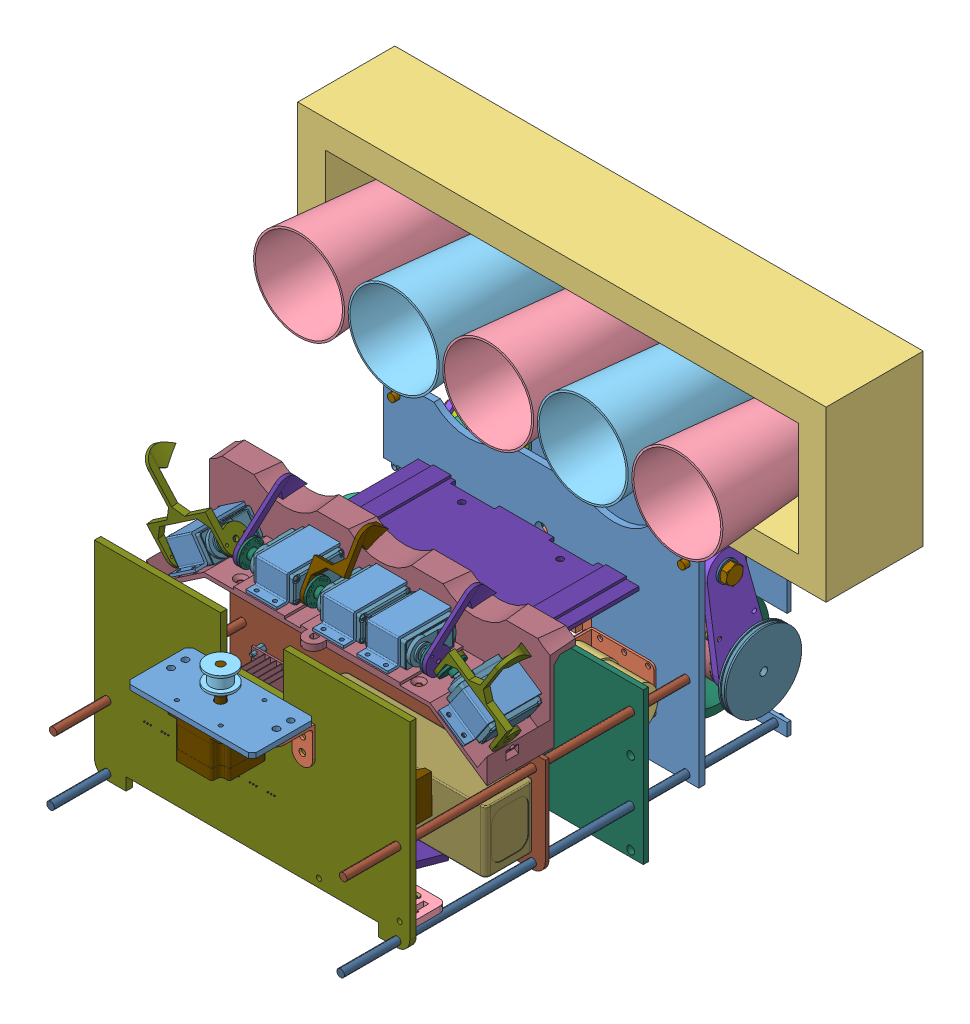
SolidWorks assembly Assemblage ROBOT SGHIR, configuration Default. Lengths in mm.
Overall size (419 329.19 386.9).
345 component instances, 73 part files, 218 mates.
Components (placement in the parent):
- baseee-1: baseee [Défaut] at (-18.9013 250.2954 189.5605) size (250 160 3)
- support_roulement-1: support_roulement [Défaut] at (62.0987 90.2954 212.5605) x (0 -1 0) z (1 0 0) size (45 40 8)
- support_roulement-2: support_roulement [Défaut] at (103.4987 90.2954 212.5605) x (0 1 0) z (-1 0 0) size (45 40 8)
- support_roulement-3: support_roulement [Défaut] at (150.0987 90.2954 212.5605) x (0 1 0) z (-1 0 0) size (45 40 8)
- support_roulement-4: support_roulement [Défaut] at (108.6987 90.2954 212.5605) x (0 1 0) z (1 0 0) size (45 40 8)
- roulement-1: roulement [Default] at (148.0987 90.2954 212.5605) x (0 0.989363 -0.145468) z (0 0.145468 0.989363) size (19 6 19)
- roulement-2: roulement [Default] at (116.6987 90.2954 212.5605) x (0 0.988428 -0.151694) z (0 0.151694 0.988428) size (19 6 19)
- roulement-3: roulement [Default] at (101.4987 90.2954 212.5605) x (0 0.989363 -0.145468) z (0 0.145468 0.989363) size (19 6 19)
- roulement-4: roulement [Default] at (70.0987 90.2954 212.5605) x (0 0.999601 -0.02823) z (0 0.02823 0.999601) size (19 6 19)
- axe de tombour-1: axe de tombour [Default] at (93.6516 90.2954 212.5605) x (0 -0.99338 -0.114871) z (-1 0 0) size (6 6 40)
- small_roue-1: small_roue [Défaut] at (80.1798 90.2954 212.5605) x (0 0.831954 -0.554845) z (1 0 0) size (23.1 23.1 19.4)
- axe de tombour-2: axe de tombour [Default] at (155.8668 90.2954 212.5605) x (0 -0.497154 0.867662) z (-1 0 0) size (6 6 40)
- small_roue-2: small_roue [Défaut] at (127.9937 90.2954 212.5605) x (0 0.856111 -0.516793) z (1 0 0) size (23.1 23.1 19.4)
- supportencodeur+encodeur+roue-1: supportencodeur+encodeur+roue [Default] at (226.6391 188.3182 195.4291) x (0 -1 0) z (-1 0 0) size (127.24 70.21 65.9)
  - Part1-1: Part1 [Default] at (40.5228 47.1314 27.8404) size (50 50 15)
  - axe-1: axe [Default] at (27.5228 27.1314 13.8404) x (0 0 -1) z (0.012333 0.999924 0) size (50 24 24)
  - levier-1: levier [Default] at (96.1154 13.1656 13.8404) x (0.979895 -0.199512 0) z (0 0 1) size (105 40 5)
  - hex screw gradeab fine_iso-1: hex screw gradeab fine_iso [ISO 8676 - M8x1.0 x 16-N] at (27.5228 27.1314 6.9404) x (0 0 1) z (0.127551 -0.991832 0) size (21.3 15.01 13)
  - plain washer normal grade a_iso-1: plain washer normal grade a_iso [Washer ISO 7089 - 8] at (27.5228 27.1314 13.8404) x (0 0 1) z (-0.997361 0.072597 0) size (1.6 16 16)
  - socket head cap screw_iso-5: socket head cap screw_iso [ISO 4762 M3 x 8 - 8N] at (27.7694 47.1299 22.3404) x (-0.012333 -0.999924 0) z (-0.32391 0.003995 0.946079) size (11 5.5 5.5)
  - socket head cap screw_iso-6: socket head cap screw_iso [ISO 4762 M3 x 8 - 8N] at (7.5243 27.3781 22.3404) x (0.999924 -0.012333 0) z (0.005971 0.484095 0.874995) size (11 5.5 5.5)
  - slotted pan head screw_iso-1: slotted pan head screw_iso [ISO 1580 - M4 x 5 - 5N] at (72.2121 32.4102 22.2404) x (0 0 -1) z (-0.691437 -0.722437 0) size (7.47 8 8)
  - Encodeur TR-1: Encodeur TR [Défaut] at (96.1154 13.1656 54.4404) x (0.979895 -0.199512 0) z (0 0 -1) size (37.8 37.8 52.6)
  - Roue Encodeur-1: Roue Encodeur [Défaut] at (96.1154 13.1656 3.9404) x (0 0 -1) z (-0.130263 -0.99148 0) size (14 60 60)
  - socket head cap screw_iso-7: socket head cap screw_iso [ISO 4762 M4 x 30 - 20N] at (14.9228 40.1314 35.4102) x (1 0 0) z (0 -0.701601 -0.71257) size (34 7 7)
- Tombour-1: Tombour [Défaut] at (165.0768 90.2954 212.5605) x (-1 0 0) z (0 0.352359 -0.935865) size (40 84.84 84.84)
- Motor Cople-1: Motor Cople [Predeterminado] at (152.8668 90.2954 212.5605) x (0 0 1) z (-1 0 0) size (25.4 25.4 9.21)
- Tombour + levier gauche-2: Tombour + levier gauche [Défaut] at (130.7568 41.7681 187.0189) x (-1 0 0) z (0 1 0) size (65.9 83.26 124.85)
  - supportencodeur+encodeur+roue-1: supportencodeur+encodeur+roue [Default] at (145.1984 8.4101 91.5046) x (0 0 1) z (-1 0 0) size (124.85 83.26 65.9) (flexible)
    - Part1-1: Part1 [Default] at (40.5228 47.1314 27.8404) size (50 50 15)
    - axe-1: axe [Default] at (27.5228 27.1314 13.8404) x (0 0 -1) z (0.999994 0.003586 0) size (50 24 24)
    - levier-1: levier [Default] at (-37.9241 2.2978 13.8404) x (-0.934955 -0.354766 0) z (0 0 1) size (105 40 5)
    - hex screw gradeab fine_iso-1: hex screw gradeab fine_iso [ISO 8676 - M8x1.0 x 16-N] at (27.5228 27.1314 6.9404) x (0 0 1) z (0.924079 -0.382202 0) size (21.3 15.01 13)
    - plain washer normal grade a_iso-1: plain washer normal grade a_iso [Washer ISO 7089 - 8] at (27.5228 27.1314 13.8404) x (0 0 1) z (-0.973268 0.229671 0) size (1.6 16 16)
    - socket head cap screw_iso-5: socket head cap screw_iso [ISO 4762 M3 x 8 - 8N] at (47.5226 27.2031 22.3404) x (-0.999994 -0.003586 0) z (-0.003073 0.857033 -0.515253) size (11 5.5 5.5)
    - socket head cap screw_iso-6: socket head cap screw_iso [ISO 4762 M3 x 8 - 8N] at (27.451 47.1313 22.3404) x (0.003586 -0.999994 0) z (0.889754 0.00319 0.45643) size (11 5.5 5.5)
    - slotted pan head screw_iso-1: slotted pan head screw_iso [ISO 1580 - M4 x 5 - 5N] at (-7.4369 -1.2027 22.2404) x (0 0 -1) z (0.467296 0.884101 0) size (7.47 8 8)
    - Encodeur TR-1: Encodeur TR [Défaut] at (-37.9241 2.2978 54.4404) x (-0.934955 -0.354766 0) z (0 0 -1) size (37.8 37.8 52.6)
    - Roue Encodeur-1: Roue Encodeur [Défaut] at (-37.9241 2.2978 3.9404) x (0 0 -1) z (0.159731 -0.987161 0) size (14 60 60)
    - socket head cap screw_iso-7: socket head cap screw_iso [ISO 4762 M4 x 30 - 20N] at (14.9228 40.1314 35.4102) x (1 0 0) z (0 -0.489793 0.871839) size (34 7 7)
- Tombour-2: Tombour [Défaut] at (47.3307 90.2954 212.5605) x (1 0 0) z (0 -0.872139 0.489257) size (40 84.84 84.84)
- accouplement moteur-1: accouplement moteur [Défaut] at (50.3307 90.2954 212.5605) size (9 25 25)
- scroll 04-1: scroll 04 [Défaut] at (77.2489 172.6222 180.1625) x (-0.291584 0.956545 0) z (0 0 1) size (20.32 14.73 13.46)
- etage moutourat-1: etage moutourat [Défaut] at (-18.9013 200.2954 257.5605) size (250 160 5)
- moteurKacem+support-1: moteurKacem+support [Default] at (34.6337 134.2418 250.1858) x (1 0 0) z (0 -1 0) size (79.5 40.7 38)
  - supportMoteur-1: supportMoteur [Default] at (29.6651 14.0747 22.9463) size (51 40.7 38)
  - moteurKacem-1: moteurKacem [Default] at (5.9651 33.0886 41.927) x (-1 0 0) z (0 -0.002768 -0.999996) size (79.5 37 37)
- support servo allu-2: support servo allu [Default] at (0.5987 137.4885 257.5605) x (1 0 0) z (0 1 0) size (80 24 5)
- moteurKacem+support-2: moteurKacem+support [Default] at (177.5638 47.8491 250.1858) x (-1 0 0) z (0 1 0) size (79.5 40.7 38)
  - supportMoteur-1: supportMoteur [Default] at (29.6651 14.0747 22.9463) size (51 40.7 38)
  - moteurKacem-1: moteurKacem [Default] at (5.9651 33.0886 41.927) x (-1 0 0) z (0 -0.002768 -0.999996) size (79.5 37 37)
- ServoAttacment2-1: ServoAttacment2 [Varsayılan] at (31.0987 127.0525 248.5605) x (0.695152 0 0.718863) z (0 -1 0) size (14 25.75 6.08)
- bras manche a air-1: bras manche a air [Default] at (28.9422 121.0525 250.6459) x (-0.718863 0 0.695152) z (0 1 0) size (80 30 4)
- small_roue-3: small_roue [Défaut] at (132.8487 89.7954 276.2744) x (0 0.856111 -0.516793) z (1 0 0) size (23.1 23.1 19.4)
- small_roue-4: small_roue [Défaut] at (79.3487 92.2954 276.2744) x (0 0.830482 -0.557045) z (-1 0 0) size (23.1 23.1 19.4)
- vis fixation tambour-1: vis fixation tambour [Default] at (66.0987 72.7954 257.5605) x (1 0 0) z (0 1 0) size (5 69.8 5)
- vis fixation tambour-2: vis fixation tambour [Default] at (66.0987 107.7954 257.5605) x (1 0 0) z (0 1 0) size (5 69.8 5)
- vis fixation tambour-3: vis fixation tambour [Default] at (99.4987 72.7954 257.5605) x (1 0 0) z (0 1 0) size (5 69.8 5)
- vis fixation tambour-4: vis fixation tambour [Default] at (99.4987 107.7954 257.5605) x (1 0 0) z (0 1 0) size (5 69.8 5)
- ressort-1: ressort [Default] at (64.5295 107.7954 230.9339) size (4.4 5.08 25.07)
- ressort-2: ressort [Default] at (97.9295 107.8027 231.9339) x (0.999989 -0.004615 0) z (0 0 1) size (4.4 5.08 25.07)
- ressort-3: ressort [Default] at (97.9295 72.8027 231.9339) x (0.999989 -0.004615 0) z (0 0 1) size (4.4 5.08 25.07)
- ressort-4: ressort [Default] at (64.5295 72.7954 235.9339) size (4.4 5.08 25.07)
- ressort-5: ressort [Default] at (111.1295 72.8027 231.9339) x (0.999989 -0.004615 0) z (0 0 1) size (4.4 5.08 25.07)
- vis fixation tambour-5: vis fixation tambour [Default] at (112.6987 107.7954 257.5605) x (1 0 0) z (0 1 0) size (5 69.8 5)
- vis fixation tambour-6: vis fixation tambour [Default] at (112.6987 72.7954 257.5605) x (1 0 0) z (0 1 0) size (5 69.8 5)
- vis fixation tambour-7: vis fixation tambour [Default] at (146.0987 72.7954 257.5605) x (1 0 0) z (0 1 0) size (5 69.8 5)
- vis fixation tambour-8: vis fixation tambour [Default] at (146.0987 107.7954 257.5605) x (1 0 0) z (0 1 0) size (5 69.8 5)
- ressort-6: ressort [Default] at (113.6444 106.5431 231.9339) x (-0.602601 0.798042 0) z (0 0 1) size (4.4 5.08 25.07)
- ressort-7: ressort [Default] at (147.0444 106.5431 231.9339) x (-0.602601 0.798042 0) z (0 0 1) size (4.4 5.08 25.07)
- ressort-8: ressort [Default] at (147.0444 71.5431 231.9339) x (-0.602601 0.798042 0) z (0 0 1) size (4.4 5.08 25.07)
- salim écrou-1: salim écrou [Défaut] at (65.7102 107.8336 251.7883) x (-0.68705 0.72661 0) z (0 0 1) size (5.79 5.76 11.17)
- rondelle-1: rondelle [Default] at (66.0987 107.7954 253.0605) size (9 9 0.5)
- 3 etage-1: 3 etage [Default] at (-18.9013 120.2954 381.2939) size (250 80 3)
- Lipot 5000 mAh-1: Lipot 5000 mAh [Default] at (153.6734 75.7626 399.2939) size (150 49 39)
- L298N Motor Driver-1: L298N Motor Driver [Default] at (26.3982 67.0454 389.2939) x (-1 0 0) z (0 1 0) size (43.5 26 43.5)
- entretoise-1: entretoise [Default] at (7.5152 85.7854 389.2939) x (0 0 -1) z (0.075316 -0.99716 0) size (10.06 5.77 5)
- entretoise-2: entretoise [Default] at (45.0327 48.3621 389.2939) x (0 0 -1) z (-0.5 -0.866025 0) size (10.06 5.77 5)
- entretoise-3: entretoise [Default] at (7.7636 48.3621 389.2939) x (0 0 -1) z (-0.5 0.866025 0) size (10.06 5.77 5)
- entretoise-4: entretoise [Default] at (45.0152 85.7854 389.2939) x (0 0 -1) z (0.075316 -0.99716 0) size (10.06 5.77 5)
- étage servo-1: étage servo [Default] at (-18.9013 129.7933 302.5605) size (250 120 4)
- etage electro-1: etage electro [Défaut] at (231.0987 40.2954 486.706) x (-1 0 0) z (0 0 1) size (250 160 5)
- support servo allu-3: support servo allu [Default] at (170.5987 56.9278 486.706) x (1 0 0) z (0 1 0) size (80 24 5)
- 3alam-1: 3alam [Défaut] at (66.7107 40.2954 431.5663) x (0.357807 0 -0.933796) z (0 1 0) size (60 150 5)
- ServoAttacment2-3: ServoAttacment2 [Varsayılan] at (201.0987 47.2954 477.706) x (-0.357807 0 0.933796) z (0 -1 0) size (14 25.75 6.08)
- TB6560 Stepper driver-1: TB6560 Stepper driver [Default] at (173.9926 122.1069 469.706) x (-0.019439 0.999811 0) z (0.999811 0.019439 0) size (50 34 75)
- Carte 8 servos.STEP-1: Carte 8 servos.STEP [Default] at (127.4764 76.1908 483.471) x (-1 0 0) z (0 0 -1) size (135 60 28.62)
  - U1.STEP-1: U1.STEP [Default] at (2.3 7.3 0.775) x (0 -1 0) z (0 0 1) size (7.62 7.92 7.75)
    - Open CASCADE STEP translator 6.8 2.2.1.STEP-1: Open CASCADE STEP translator 6.8 2.2.1.STEP [Default] at origin size (7.62 7.92 7.75)
      - Body_1.STEP-1: Body_1.STEP [Default] at (2.5 4 0) x (0 1 0) z (1 0 0) size (7.92 7.75 7.62)
  - U2.STEP-1: U2.STEP [Default] at (16.56 8.1 0.775) x (0 -1 0) z (0 0 1) size (7.62 7.92 7.75)
    - Open CASCADE STEP translator 6.8 2.3.1.STEP-1: Open CASCADE STEP translator 6.8 2.3.1.STEP [Default] at origin size (7.62 7.92 7.75)
      - Body_1.STEP-1: Body_1.STEP [Default] at (2.5 4 0) x (0 1 0) z (1 0 0) size (7.92 7.75 7.62)
  - U3.STEP-1: U3.STEP [Default] at (30.3 7.8 0.775) x (0 -1 0) z (0 0 1) size (7.62 7.92 7.75)
    - Open CASCADE STEP translator 6.8 2.4.1.STEP-1: Open CASCADE STEP translator 6.8 2.4.1.STEP [Default] at origin size (7.62 7.92 7.75)
      - Body_1.STEP-1: Body_1.STEP [Default] at (2.5 4 0) x (0 1 0) z (1 0 0) size (7.92 7.75 7.62)
  - U4.STEP-1: U4.STEP [Default] at (44.2 7.6 0.775) x (0 -1 0) z (0 0 1) size (7.62 7.92 7.75)
    - Open CASCADE STEP translator 6.8 2.5.1.STEP-1: Open CASCADE STEP translator 6.8 2.5.1.STEP [Default] at origin size (7.62 7.92 7.75)
      - Body_1.STEP-1: Body_1.STEP [Default] at (2.5 4 0) x (0 1 0) z (1 0 0) size (7.92 7.75 7.62)
  - J2.STEP-1: J2.STEP [Default] at (9.1 -11.4 0.775) x (-1 0 0) z (0 0 1) size (6 2 8.8)
    - Open CASCADE STEP translator 6.8 2.6.1.STEP-1: Open CASCADE STEP translator 6.8 2.6.1.STEP [Default] at origin size (6 2 8.8)
      - Body_1-0.STEP-1: Body_1-0.STEP [Default] at (1.5 -1 -3) x (0 1 0) z (1 0 0) size (2 8.8 6)
        - Carte 8 servos-prt1.STEP-1: Carte 8 servos-prt1.STEP [Default] at origin size (2 8.8 2)
        - Carte 8 servos-prt2.STEP-1: Carte 8 servos-prt2.STEP [Default] at origin size (2 8.8 2)
        - Carte 8 servos-prt3.STEP-1: Carte 8 servos-prt3.STEP [Default] at origin size (2 8.8 2)
  - J3.STEP-1: J3.STEP [Default] at (22.86 -11.3 0.775) x (-1 0 0) z (0 0 1) size (6 2 8.8)
    - Open CASCADE STEP translator 6.8 2.7.1.STEP-1: Open CASCADE STEP translator 6.8 2.7.1.STEP [Default] at origin size (6 2 8.8)
      - Body_1-0.STEP-1: Body_1-0.STEP [Default] at (1.5 -1 -3) x (0 1 0) z (1 0 0) size (2 8.8 6)
        - Carte 8 servos-prt1.STEP-1: Carte 8 servos-prt1.STEP [Default] at origin size (2 8.8 2)
        - Carte 8 servos-prt2.STEP-1: Carte 8 servos-prt2.STEP [Default] at origin size (2 8.8 2)
        - Carte 8 servos-prt3.STEP-1: Carte 8 servos-prt3.STEP [Default] at origin size (2 8.8 2)
  - J4.STEP-1: J4.STEP [Default] at (36.8 -11.3 0.775) x (-1 0 0) z (0 0 1) size (6 2 8.8)
    - Open CASCADE STEP translator 6.8 2.8.1.STEP-1: Open CASCADE STEP translator 6.8 2.8.1.STEP [Default] at origin size (6 2 8.8)
      - Body_1-0.STEP-1: Body_1-0.STEP [Default] at (1.5 -1 -3) x (0 1 0) z (1 0 0) size (2 8.8 6)
        - Carte 8 servos-prt1.STEP-1: Carte 8 servos-prt1.STEP [Default] at origin size (2 8.8 2)
        - Carte 8 servos-prt2.STEP-1: Carte 8 servos-prt2.STEP [Default] at origin size (2 8.8 2)
        - Carte 8 servos-prt3.STEP-1: Carte 8 servos-prt3.STEP [Default] at origin size (2 8.8 2)
  - J5.STEP-1: J5.STEP [Default] at (50.7 -11.3 0.775) x (-1 0 0) z (0 0 1) size (6 2 8.8)
    - Open CASCADE STEP translator 6.8 2.9.1.STEP-1: Open CASCADE STEP translator 6.8 2.9.1.STEP [Default] at origin size (6 2 8.8)
      - Body_1-0.STEP-1: Body_1-0.STEP [Default] at (1.5 -1 -3) x (0 1 0) z (1 0 0) size (2 8.8 6)
        - Carte 8 servos-prt1.STEP-1: Carte 8 servos-prt1.STEP [Default] at origin size (2 8.8 2)
        - Carte 8 servos-prt2.STEP-1: Carte 8 servos-prt2.STEP [Default] at origin size (2 8.8 2)
        - Carte 8 servos-prt3.STEP-1: Carte 8 servos-prt3.STEP [Default] at origin size (2 8.8 2)
  - J6.STEP-1: J6.STEP [Default] at (-4.8 19.8 0.775) x (-1 0 0) z (0 0 1) size (10 7.5 13.25)
    - Open CASCADE STEP translator 6.8 2.10.1.STEP-1: Open CASCADE STEP translator 6.8 2.10.1.STEP [Default] at origin size (10 7.5 13.25)
      - Body_1-1.STEP-1: Body_1-1.STEP [Default] at (7.5 4 0) x (-1 0 0) z (0 1 0) size (10 13.25 7.5)
  - C1.STEP-1: C1.STEP [Default] at (-5.9 9.4 0.775) x (-1 0 0) z (0 0 1) size (6.31 6.3 13.91)
    - Open CASCADE STEP translator 6.8 2.11.1.STEP-1: Open CASCADE STEP translator 6.8 2.11.1.STEP [Default] at origin size (6.31 6.3 13.91)
      - Body_1-2.STEP-1: Body_1-2.STEP [Default] at (1.25 0 0) x (1 0 0) z (0 -1 0) size (6.31 13.91 6.3)
  - C9.STEP-1: C9.STEP [Default] at (7.54 -3.5 0.775) x (-1 0 0) z (0 0 1) size (6.31 6.3 13.91)
    - Open CASCADE STEP translator 6.8 2.12.1.STEP-1: Open CASCADE STEP translator 6.8 2.12.1.STEP [Default] at origin size (6.31 6.3 13.91)
      - Body_1-2.STEP-1: Body_1-2.STEP [Default] at (1.25 0 0) x (1 0 0) z (0 -1 0) size (6.31 13.91 6.3)
  - C10.STEP-1: C10.STEP [Default] at (21.36 -2.9 0.775) x (-1 0 0) z (0 0 1) size (6.31 6.3 13.91)
    - Open CASCADE STEP translator 6.8 2.13.1.STEP-1: Open CASCADE STEP translator 6.8 2.13.1.STEP [Default] at origin size (6.31 6.3 13.91)
      - Body_1-2.STEP-1: Body_1-2.STEP [Default] at (1.25 0 0) x (1 0 0) z (0 -1 0) size (6.31 13.91 6.3)
  - C11.STEP-1: C11.STEP [Default] at (35.5 -2.8 0.775) x (-1 0 0) z (0 0 1) size (6.31 6.3 13.91)
    - Open CASCADE STEP translator 6.8 2.14.1.STEP-1: Open CASCADE STEP translator 6.8 2.14.1.STEP [Default] at origin size (6.31 6.3 13.91)
      - Body_1-2.STEP-1: Body_1-2.STEP [Default] at (1.25 0 0) x (1 0 0) z (0 -1 0) size (6.31 13.91 6.3)
  - C12.STEP-1: C12.STEP [Default] at (49.2 -3 0.775) x (-1 0 0) z (0 0 1) size (6.31 6.3 13.91)
    - Open CASCADE STEP translator 6.8 2.15.1.STEP-1: Open CASCADE STEP translator 6.8 2.15.1.STEP [Default] at origin size (6.31 6.3 13.91)
      - Body_1-2.STEP-1: Body_1-2.STEP [Default] at (1.25 0 0) x (1 0 0) z (0 -1 0) size (6.31 13.91 6.3)
  - R1.STEP-1: R1.STEP [Default] at (11.2 11.3 0.775) x (-1 0 0) z (0 0 1) size (10.82 1.37 5.33)
    - Open CASCADE STEP translator 6.8 2.16.1.STEP-1: Open CASCADE STEP translator 6.8 2.16.1.STEP [Default] at origin size (10.82 1.37 5.33)
      - Body_1-3.STEP-1: Body_1-3.STEP [Default] at origin size (5.08 1.37 1.37)
      - Pin_1.STEP-1: Pin_1.STEP [Default] at origin size (3.2 0.66 4.98)
      - Pin_2.STEP-1: Pin_2.STEP [Default] at (20.32 0 0) x (-1 0 0) z (0 0 1) size (3.2 0.66 4.98)
  - R2.STEP-1: R2.STEP [Default] at (25.16 11.3 0.775) x (-1 0 0) z (0 0 1) size (10.82 1.37 5.33)
    - Open CASCADE STEP translator 6.8 2.16.1.STEP-1: Open CASCADE STEP translator 6.8 2.16.1.STEP [Default] at origin size (10.82 1.37 5.33)
      - Body_1-3.STEP-1: Body_1-3.STEP [Default] at origin size (5.08 1.37 1.37)
      - Pin_1.STEP-1: Pin_1.STEP [Default] at origin size (3.2 0.66 4.98)
      - Pin_2.STEP-1: Pin_2.STEP [Default] at (20.32 0 0) x (-1 0 0) z (0 0 1) size (3.2 0.66 4.98)
  - R3.STEP-1: R3.STEP [Default] at (28.8 11 0.775) size (10.82 1.37 5.33)
    - Open CASCADE STEP translator 6.8 2.16.1.STEP-1: Open CASCADE STEP translator 6.8 2.16.1.STEP [Default] at origin size (10.82 1.37 5.33)
      - Body_1-3.STEP-1: Body_1-3.STEP [Default] at origin size (5.08 1.37 1.37)
      - Pin_1.STEP-1: Pin_1.STEP [Default] at origin size (3.2 0.66 4.98)
      - Pin_2.STEP-1: Pin_2.STEP [Default] at (20.32 0 0) x (-1 0 0) z (0 0 1) size (3.2 0.66 4.98)
  - R4.STEP-1: R4.STEP [Default] at (53.56 11.6 0.775) x (-1 0 0) z (0 0 1) size (10.82 1.37 5.33)
    - Open CASCADE STEP translator 6.8 2.16.1.STEP-1: Open CASCADE STEP translator 6.8 2.16.1.STEP [Default] at origin size (10.82 1.37 5.33)
      - Body_1-3.STEP-1: Body_1-3.STEP [Default] at origin size (5.08 1.37 1.37)
      - Pin_1.STEP-1: Pin_1.STEP [Default] at origin size (3.2 0.66 4.98)
      - Pin_2.STEP-1: Pin_2.STEP [Default] at (20.32 0 0) x (-1 0 0) z (0 0 1) size (3.2 0.66 4.98)
  - U6.STEP-1: U6.STEP [Default] at (48.34 19.4 0.775) size (9.97 4.45 28.62)
    - Open CASCADE STEP translator 6.8 2.20.1.STEP-1: Open CASCADE STEP translator 6.8 2.20.1.STEP [Default] at origin size (9.97 4.45 28.62)
      - Body_1-4.STEP-1: Body_1-4.STEP [Default] at (0 3 3.5) x (1 0 0) z (0 -1 0) size (9.97 28.62 4.45)
  - U7.STEP-1: U7.STEP [Default] at (20.1 19.4 0.775) size (9.97 4.45 28.62)
    - Open CASCADE STEP translator 6.8 2.21.1.STEP-1: Open CASCADE STEP translator 6.8 2.21.1.STEP [Default] at origin size (9.97 4.45 28.62)
      - Body_1-4.STEP-1: Body_1-4.STEP [Default] at (0 3 3.5) x (1 0 0) z (0 -1 0) size (9.97 28.62 4.45)
  - U8.STEP-1: U8.STEP [Default] at (34.14 19.2 0.775) size (9.97 4.45 28.62)
    - Open CASCADE STEP translator 6.8 2.22.1.STEP-1: Open CASCADE STEP translator 6.8 2.22.1.STEP [Default] at origin size (9.97 4.45 28.62)
      - Body_1-4.STEP-1: Body_1-4.STEP [Default] at (0 3 3.5) x (1 0 0) z (0 -1 0) size (9.97 28.62 4.45)
  - U5.STEP-1: U5.STEP [Default] at (5.9 19.8 0.775) size (9.97 4.45 28.62)
    - Open CASCADE STEP translator 6.8 2.23.1.STEP-1: Open CASCADE STEP translator 6.8 2.23.1.STEP [Default] at origin size (9.97 4.45 28.62)
      - Body_1-4.STEP-1: Body_1-4.STEP [Default] at (0 3 3.5) x (1 0 0) z (0 -1 0) size (9.97 28.62 4.45)
  - D1.STEP-1: D1.STEP [Default] at (0.84 15.5 0.775) size (11.02 2.72 5.32)
    - Open CASCADE STEP translator 6.8 2.24.1.STEP-1: Open CASCADE STEP translator 6.8 2.24.1.STEP [Default] at origin size (11.02 2.72 5.32)
      - Body_1-5.STEP-1: Body_1-5.STEP [Default] at (10.1 0 0) size (11.02 2.72 5.32)
  - D2.STEP-1: D2.STEP [Default] at (15.4 15.3 0.775) size (11.02 2.72 5.32)
    - Open CASCADE STEP translator 6.8 2.25.1.STEP-1: Open CASCADE STEP translator 6.8 2.25.1.STEP [Default] at origin size (11.02 2.72 5.32)
      - Body_1-5.STEP-1: Body_1-5.STEP [Default] at (10.1 0 0) size (11.02 2.72 5.32)
  - D4.STEP-1: D4.STEP [Default] at (43 15.3 0.775) size (11.02 2.72 5.32)
    - Open CASCADE STEP translator 6.8 2.26.1.STEP-1: Open CASCADE STEP translator 6.8 2.26.1.STEP [Default] at origin size (11.02 2.72 5.32)
      - Body_1-5.STEP-1: Body_1-5.STEP [Default] at (10.1 0 0) size (11.02 2.72 5.32)
  - D3.STEP-1: D3.STEP [Default] at (29.24 15 0.775) size (11.02 2.72 5.32)
    - Open CASCADE STEP translator 6.8 2.27.1.STEP-1: Open CASCADE STEP translator 6.8 2.27.1.STEP [Default] at origin size (11.02 2.72 5.32)
      - Body_1-5.STEP-1: Body_1-5.STEP [Default] at (10.1 0 0) size (11.02 2.72 5.32)
  - U13.STEP-1: U13.STEP [Default] at (61.94 19.4 0.775) size (9.97 4.45 28.62)
    - Open CASCADE STEP translator 6.8 2.28.1.STEP-1: Open CASCADE STEP translator 6.8 2.28.1.STEP [Default] at origin size (9.97 4.45 28.62)
      - Body_1-4.STEP-1: Body_1-4.STEP [Default] at (0 3 3.5) x (1 0 0) z (0 -1 0) size (9.97 28.62 4.45)
  - U14.STEP-1: U14.STEP [Default] at (75.94 19.4 0.775) size (9.97 4.45 28.62)
    - Open CASCADE STEP translator 6.8 2.29.1.STEP-1: Open CASCADE STEP translator 6.8 2.29.1.STEP [Default] at origin size (9.97 4.45 28.62)
      - Body_1-4.STEP-1: Body_1-4.STEP [Default] at (0 3 3.5) x (1 0 0) z (0 -1 0) size (9.97 28.62 4.45)
  - U16.STEP-1: U16.STEP [Default] at (90.04 19.3 0.775) size (9.97 4.45 28.62)
    - Open CASCADE STEP translator 6.8 2.30.1.STEP-1: Open CASCADE STEP translator 6.8 2.30.1.STEP [Default] at origin size (9.97 4.45 28.62)
      - Body_1-4.STEP-1: Body_1-4.STEP [Default] at (0 3 3.5) x (1 0 0) z (0 -1 0) size (9.97 28.62 4.45)
  - U15.STEP-1: U15.STEP [Default] at (103.94 19.2 0.775) size (9.97 4.45 28.62)
    - Open CASCADE STEP translator 6.8 2.31.1.STEP-1: Open CASCADE STEP translator 6.8 2.31.1.STEP [Default] at origin size (9.97 4.45 28.62)
      - Body_1-4.STEP-1: Body_1-4.STEP [Default] at (0 3 3.5) x (1 0 0) z (0 -1 0) size (9.97 28.62 4.45)
  - D8.STEP-1: D8.STEP [Default] at (57.3 15.2 0.775) size (11.02 2.72 5.32)
    - Open CASCADE STEP translator 6.8 2.32.1.STEP-1: Open CASCADE STEP translator 6.8 2.32.1.STEP [Default] at origin size (11.02 2.72 5.32)
      - Body_1-5.STEP-1: Body_1-5.STEP [Default] at (10.1 0 0) size (11.02 2.72 5.32)
  - U9.STEP-1: U9.STEP [Default] at (58.8 7.9 0.775) x (0 -1 0) z (0 0 1) size (7.62 7.92 7.75)
    - Open CASCADE STEP translator 6.8 2.33.1.STEP-1: Open CASCADE STEP translator 6.8 2.33.1.STEP [Default] at origin size (7.62 7.92 7.75)
      - Body_1.STEP-1: Body_1.STEP [Default] at (2.5 4 0) x (0 1 0) z (1 0 0) size (7.92 7.75 7.62)
  - R5.STEP-1: R5.STEP [Default] at (57.3 11.4 0.775) size (10.82 1.37 5.33)
    - Open CASCADE STEP translator 6.8 2.16.1.STEP-1: Open CASCADE STEP translator 6.8 2.16.1.STEP [Default] at origin size (10.82 1.37 5.33)
      - Body_1-3.STEP-1: Body_1-3.STEP [Default] at origin size (5.08 1.37 1.37)
      - Pin_1.STEP-1: Pin_1.STEP [Default] at origin size (3.2 0.66 4.98)
      - Pin_2.STEP-1: Pin_2.STEP [Default] at (20.32 0 0) x (-1 0 0) z (0 0 1) size (3.2 0.66 4.98)
  - C2.STEP-1: C2.STEP [Default] at (64.04 -2.9 0.775) x (-1 0 0) z (0 0 1) size (6.31 6.3 13.91)
    - Open CASCADE STEP translator 6.8 2.35.1.STEP-1: Open CASCADE STEP translator 6.8 2.35.1.STEP [Default] at origin size (6.31 6.3 13.91)
      - Body_1-2.STEP-1: Body_1-2.STEP [Default] at (1.25 0 0) x (1 0 0) z (0 -1 0) size (6.31 13.91 6.3)
  - J7.STEP-1: J7.STEP [Default] at (65.5 -11.3 0.775) x (-1 0 0) z (0 0 1) size (6 2 8.8)
    - Open CASCADE STEP translator 6.8 2.36.1.STEP-1: Open CASCADE STEP translator 6.8 2.36.1.STEP [Default] at origin size (6 2 8.8)
      - Body_1-0.STEP-1: Body_1-0.STEP [Default] at (1.5 -1 -3) x (0 1 0) z (1 0 0) size (2 8.8 6)
        - Carte 8 servos-prt1.STEP-1: Carte 8 servos-prt1.STEP [Default] at origin size (2 8.8 2)
        - Carte 8 servos-prt2.STEP-1: Carte 8 servos-prt2.STEP [Default] at origin size (2 8.8 2)
        - Carte 8 servos-prt3.STEP-1: Carte 8 servos-prt3.STEP [Default] at origin size (2 8.8 2)
  - D5.STEP-1: D5.STEP [Default] at (99.4 14.7 0.775) size (11.02 2.72 5.32)
    - Open CASCADE STEP translator 6.8 2.37.1.STEP-1: Open CASCADE STEP translator 6.8 2.37.1.STEP [Default] at origin size (11.02 2.72 5.32)
      - Body_1-5.STEP-1: Body_1-5.STEP [Default] at (10.1 0 0) size (11.02 2.72 5.32)
  - D6.STEP-1: D6.STEP [Default] at (85.1 14.8 0.775) size (11.02 2.72 5.32)
    - Open CASCADE STEP translator 6.8 2.38.1.STEP-1: Open CASCADE STEP translator 6.8 2.38.1.STEP [Default] at origin size (11.02 2.72 5.32)
      - Body_1-5.STEP-1: Body_1-5.STEP [Default] at (10.1 0 0) size (11.02 2.72 5.32)
  - D7.STEP-1: D7.STEP [Default] at (71.24 14.8 0.775) size (11.02 2.72 5.32)
    - Open CASCADE STEP translator 6.8 2.39.1.STEP-1: Open CASCADE STEP translator 6.8 2.39.1.STEP [Default] at origin size (11.02 2.72 5.32)
      - Body_1-5.STEP-1: Body_1-5.STEP [Default] at (10.1 0 0) size (11.02 2.72 5.32)
  - R6.STEP-1: R6.STEP [Default] at (71.4 11.4 0.775) size (10.82 1.37 5.33)
    - Open CASCADE STEP translator 6.8 2.16.1.STEP-1: Open CASCADE STEP translator 6.8 2.16.1.STEP [Default] at origin size (10.82 1.37 5.33)
      - Body_1-3.STEP-1: Body_1-3.STEP [Default] at origin size (5.08 1.37 1.37)
      - Pin_1.STEP-1: Pin_1.STEP [Default] at origin size (3.2 0.66 4.98)
      - Pin_2.STEP-1: Pin_2.STEP [Default] at (20.32 0 0) x (-1 0 0) z (0 0 1) size (3.2 0.66 4.98)
  - R7.STEP-1: R7.STEP [Default] at (84.8 11.2 0.775) size (10.82 1.37 5.33)
    - Open CASCADE STEP translator 6.8 2.16.1.STEP-1: Open CASCADE STEP translator 6.8 2.16.1.STEP [Default] at origin size (10.82 1.37 5.33)
      - Body_1-3.STEP-1: Body_1-3.STEP [Default] at origin size (5.08 1.37 1.37)
      - Pin_1.STEP-1: Pin_1.STEP [Default] at origin size (3.2 0.66 4.98)
      - Pin_2.STEP-1: Pin_2.STEP [Default] at (20.32 0 0) x (-1 0 0) z (0 0 1) size (3.2 0.66 4.98)
  - R8.STEP-1: R8.STEP [Default] at (99.4 11.1 0.775) size (10.82 1.37 5.33)
    - Open CASCADE STEP translator 6.8 2.16.1.STEP-1: Open CASCADE STEP translator 6.8 2.16.1.STEP [Default] at origin size (10.82 1.37 5.33)
      - Body_1-3.STEP-1: Body_1-3.STEP [Default] at origin size (5.08 1.37 1.37)
      - Pin_1.STEP-1: Pin_1.STEP [Default] at origin size (3.2 0.66 4.98)
      - Pin_2.STEP-1: Pin_2.STEP [Default] at (20.32 0 0) x (-1 0 0) z (0 0 1) size (3.2 0.66 4.98)
  - U10.STEP-1: U10.STEP [Default] at (72.1 7.9 0.775) x (0 -1 0) z (0 0 1) size (7.62 7.92 7.75)
    - Open CASCADE STEP translator 6.8 2.43.1.STEP-1: Open CASCADE STEP translator 6.8 2.43.1.STEP [Default] at origin size (7.62 7.92 7.75)
      - Body_1.STEP-1: Body_1.STEP [Default] at (2.5 4 0) x (0 1 0) z (1 0 0) size (7.92 7.75 7.62)
  - C3.STEP-1: C3.STEP [Default] at (91.74 -3 0.775) x (-1 0 0) z (0 0 1) size (6.31 6.3 13.91)
    - Open CASCADE STEP translator 6.8 2.44.1.STEP-1: Open CASCADE STEP translator 6.8 2.44.1.STEP [Default] at origin size (6.31 6.3 13.91)
      - Body_1-2.STEP-1: Body_1-2.STEP [Default] at (1.25 0 0) x (1 0 0) z (0 -1 0) size (6.31 13.91 6.3)
  - J9.STEP-1: J9.STEP [Default] at (78.7 -11.1 0.775) x (-1 0 0) z (0 0 1) size (6 2 8.8)
    - Open CASCADE STEP translator 6.8 2.45.1.STEP-1: Open CASCADE STEP translator 6.8 2.45.1.STEP [Default] at origin size (6 2 8.8)
      - Body_1-0.STEP-1: Body_1-0.STEP [Default] at (1.5 -1 -3) x (0 1 0) z (1 0 0) size (2 8.8 6)
        - Carte 8 servos-prt1.STEP-1: Carte 8 servos-prt1.STEP [Default] at origin size (2 8.8 2)
        - Carte 8 servos-prt2.STEP-1: Carte 8 servos-prt2.STEP [Default] at origin size (2 8.8 2)
        - Carte 8 servos-prt3.STEP-1: Carte 8 servos-prt3.STEP [Default] at origin size (2 8.8 2)
  - U11.STEP-1: U11.STEP [Default] at (86.4 7.3 0.775) x (0 -1 0) z (0 0 1) size (7.62 7.92 7.75)
    - Open CASCADE STEP translator 6.8 2.46.1.STEP-1: Open CASCADE STEP translator 6.8 2.46.1.STEP [Default] at origin size (7.62 7.92 7.75)
      - Body_1.STEP-1: Body_1.STEP [Default] at (2.5 4 0) x (0 1 0) z (1 0 0) size (7.92 7.75 7.62)
  - U12.STEP-1: U12.STEP [Default] at (100.9 6.9 0.775) x (0 -1 0) z (0 0 1) size (7.62 7.92 7.75)
    - Open CASCADE STEP translator 6.8 2.47.1.STEP-1: Open CASCADE STEP translator 6.8 2.47.1.STEP [Default] at origin size (7.62 7.92 7.75)
      - Body_1.STEP-1: Body_1.STEP [Default] at (2.5 4 0) x (0 1 0) z (1 0 0) size (7.92 7.75 7.62)
  - C4.STEP-1: C4.STEP [Default] at (77.54 -3 0.775) x (-1 0 0) z (0 0 1) size (6.31 6.3 13.91)
    - Open CASCADE STEP translator 6.8 2.48.1.STEP-1: Open CASCADE STEP translator 6.8 2.48.1.STEP [Default] at origin size (6.31 6.3 13.91)
      - Body_1-2.STEP-1: Body_1-2.STEP [Default] at (1.25 0 0) x (1 0 0) z (0 -1 0) size (6.31 13.91 6.3)
  - C5.STEP-1: C5.STEP [Default] at (106.3 -3 0.775) x (-1 0 0) z (0 0 1) size (6.31 6.3 13.91)
    - Open CASCADE STEP translator 6.8 2.49.1.STEP-1: Open CASCADE STEP translator 6.8 2.49.1.STEP [Default] at origin size (6.31 6.3 13.91)
      - Body_1-2.STEP-1: Body_1-2.STEP [Default] at (1.25 0 0) x (1 0 0) z (0 -1 0) size (6.31 13.91 6.3)
  - J8.STEP-1: J8.STEP [Default] at (93.6 -11 0.775) x (-1 0 0) z (0 0 1) size (6 2 8.8)
    - Open CASCADE STEP translator 6.8 2.50.1.STEP-1: Open CASCADE STEP translator 6.8 2.50.1.STEP [Default] at origin size (6 2 8.8)
      - Body_1-0.STEP-1: Body_1-0.STEP [Default] at (1.5 -1 -3) x (0 1 0) z (1 0 0) size (2 8.8 6)
        - Carte 8 servos-prt1.STEP-1: Carte 8 servos-prt1.STEP [Default] at origin size (2 8.8 2)
        - Carte 8 servos-prt2.STEP-1: Carte 8 servos-prt2.STEP [Default] at origin size (2 8.8 2)
        - Carte 8 servos-prt3.STEP-1: Carte 8 servos-prt3.STEP [Default] at origin size (2 8.8 2)
  - J10.STEP-1: J10.STEP [Default] at (107.9 -11.2 0.775) x (-1 0 0) z (0 0 1) size (6 2 8.8)
    - Open CASCADE STEP translator 6.8 2.51.1.STEP-1: Open CASCADE STEP translator 6.8 2.51.1.STEP [Default] at origin size (6 2 8.8)
      - Body_1-0.STEP-1: Body_1-0.STEP [Default] at (1.5 -1 -3) x (0 1 0) z (1 0 0) size (2 8.8 6)
        - Carte 8 servos-prt1.STEP-1: Carte 8 servos-prt1.STEP [Default] at origin size (2 8.8 2)
        - Carte 8 servos-prt2.STEP-1: Carte 8 servos-prt2.STEP [Default] at origin size (2 8.8 2)
        - Carte 8 servos-prt3.STEP-1: Carte 8 servos-prt3.STEP [Default] at origin size (2 8.8 2)
  - R9.STEP-1: R9.STEP [Default] at (-7.5 -13.4 0.775) x (0 1 0) z (0 0 1) size (10.82 1.37 5.33)
    - Open CASCADE STEP translator 6.8 2.16.1.STEP-1: Open CASCADE STEP translator 6.8 2.16.1.STEP [Default] at origin size (10.82 1.37 5.33)
      - Body_1-3.STEP-1: Body_1-3.STEP [Default] at origin size (5.08 1.37 1.37)
      - Pin_1.STEP-1: Pin_1.STEP [Default] at origin size (3.2 0.66 4.98)
      - Pin_2.STEP-1: Pin_2.STEP [Default] at (20.32 0 0) x (-1 0 0) z (0 0 1) size (3.2 0.66 4.98)
  - D9.STEP-1: D9.STEP [Default] at (-5.8 2.4 0.775) x (-1 0 0) z (0 0 1) size (5.9 5.9 15.6)
    - Open CASCADE STEP translator 6.8 2.53.1.STEP-1: Open CASCADE STEP translator 6.8 2.53.1.STEP [Default] at origin size (5.9 5.9 15.6)
      - Body_1-6.STEP-1: Body_1-6.STEP [Default] at (1.2 0 0) x (0 1 0) z (1 0 0) size (5.9 15.6 5.9)
  - J1.STEP-1: J1.STEP [Default] at (46.72 36.2 0.775) size (20 2 8.8)
    - Open CASCADE STEP translator 6.8 2.54.1.STEP-1: Open CASCADE STEP translator 6.8 2.54.1.STEP [Default] at origin size (20 2 8.8)
      - Body_1-1-7.STEP-1: Body_1-1-7.STEP [Default] at (-15.5 11 0) x (0 1 0) z (1 0 0) size (2 8.8 20)
        - Carte 8 servos-prt12.STEP-1: Carte 8 servos-prt12.STEP [Default] at (-11.7456 -3.5716 15.716) size (2 8.8 2)
        - Carte 8 servos-prt13.STEP-1: Carte 8 servos-prt13.STEP [Default] at (-11.7456 -3.5716 15.716) size (2 8.8 2)
        - Carte 8 servos-prt14.STEP-1: Carte 8 servos-prt14.STEP [Default] at (-11.7456 -3.5716 15.716) size (2 8.8 2)
        - Carte 8 servos-prt13.STEP-2: Carte 8 servos-prt13.STEP [Default] at (-11.7456 -3.5716 19.716) size (2 8.8 2)
        - Carte 8 servos-prt13.STEP-3: Carte 8 servos-prt13.STEP [Default] at (-11.7456 -3.5716 21.716) size (2 8.8 2)
        - Carte 8 servos-prt13.STEP-4: Carte 8 servos-prt13.STEP [Default] at (-11.7456 -3.5716 25.716) size (2 8.8 2)
        - Carte 8 servos-prt13.STEP-5: Carte 8 servos-prt13.STEP [Default] at (-11.7456 -3.5716 23.716) size (2 8.8 2)
        - Carte 8 servos-prt13.STEP-6: Carte 8 servos-prt13.STEP [Default] at (-11.7456 -3.5716 31.716) size (2 8.8 2)
        - Carte 8 servos-prt13.STEP-7: Carte 8 servos-prt13.STEP [Default] at (-11.7456 -3.5716 27.716) size (2 8.8 2)
        - Carte 8 servos-prt13.STEP-8: Carte 8 servos-prt13.STEP [Default] at (-11.7456 -3.5716 29.716) size (2 8.8 2)
  - Layer_1.STEP-1: Layer_1.STEP [Default] at origin size (135 60 1.55)
- base vertical-1: base vertical [Default] at (18.5987 165.1523 392.5605) x (1 0 0) z (0 -1 0) size (175 120 5)
- NEMA34-JK86HS68-5904-1: NEMA34-JK86HS68-5904 [Default] at (106.1099 167.9029 516.706) size (43.4 62.69 42.8)
- support pasàpas-1: support pasàpas [Default] at (66.0987 165.2954 541.706) x (1 0 0) z (0 -1 0) size (100 50 4)
- grand_l-1: grand_l [Défaut] at (156.0987 152.5439 492.2529) x (0 -1 0) z (-1 0 0) size (32 32 16.5)
- grand_l-2: grand_l [Défaut] at (72.5987 152.5439 492.2529) x (0 -1 0) z (-1 0 0) size (32 32 16.5)
- small_roue-5: small_roue [Défaut] at (106.0836 183.281 516.7322) x (0.991363 0 -0.131146) z (0 -1 0) size (23.1 23.1 19.4)
- eceuil-1: eceuil [Default] at (-103.4013 335.9793 169.0985) size (419 134 77)
- green cup-1: green cup [Default] at (485.3781 31.1002 232.7106) x (1 0 0) z (0 1 0) size (72.14 116.16 72.14)
- red cup-1: red cup [Default] at (410.3781 31.1002 232.7106) x (1 0 0) z (0 1 0) size (72.14 116.16 72.14)
- green cup-2: green cup [Default] at (335.3781 31.1002 232.7106) x (1 0 0) z (0 1 0) size (72.14 116.16 72.14)
- green cup-4: green cup [Default] at (635.3781 31.1002 232.7106) x (1 0 0) z (0 1 0) size (72.14 116.16 72.14)
- red cup-2: red cup [Default] at (560.3781 31.1002 232.7106) x (1 0 0) z (0 1 0) size (72.14 116.16 72.14)
- verin complet-2: verin complet [Défaut] at (90.0987 55.7529 400.2315) x (0 0 1) z (1 0 0) size (30 107 59)
  - body-1: body [Défaut] at (-78.671 0.7551 4) size (30 107 59)
- support de fixation-1: support de fixation [Default] at (110.5987 159.1523 327.5605) x (0 0 -1) z (0 -1 0) size (30 30 15)
- tige-2: tige [Défaut] at (104.5987 135.7933 321.5605) x (1 0 0) z (0 -1 0) size (13 13 72)
- tige pour palier-1: tige pour palier [Default] at (-8.9013 190.2954 186.5605) size (6 6 80)
- tige pour palier-2: tige pour palier [Default] at (221.0987 190.2954 186.5605) x (0.957173 0.289518 0) z (0 0 1) size (6 6 80)
- grand tige 350mm-1: grand tige 350mm [Default] at (221.0987 45.2954 186.5605) size (6 6 350)
- grand tige 350mm-2: grand tige 350mm [Default] at (-8.9013 45.2954 186.5605) size (6 6 350)
- tige 280mm-1: tige 280mm [Default] at (221.0987 110.2954 254.5605) size (6 6 280)
- tige 280mm-2: tige 280mm [Default] at (-8.9013 95.2954 254.5605) x (-0.985584 -0.169189 0) z (0 0 1) size (6 6 280)
- Servo noir-1: Servo noir [По умолчанию] at (191.0987 89.2954 477.706) x (-1 0 0) z (0 0 1) size (53 41.52 20)
- Servo noir-2: Servo noir [По умолчанию] at (21.0987 171.4885 248.5605) x (-1 0 0) z (0 0 1) size (53 41.52 20)
- new system-1: new system [Default] at (106.0987 167.1523 387.4162) x (-1 0 0) z (0 1 0) size (334.8 80 104.66)
  - main-1: main [Default] at origin size (270 80 71.41)
  - Servo noir pince-1: Servo noir pince [По умолчанию] at (124.6594 23 -8.665) x (0 -1 0) z (-0.561983 0 -0.827149) size (40 41.52 20)
  - ServoAttacmentround-8: ServoAttacmentround [Varsayılan] at (88.2649 33 16.0623) x (0.053507 -0.995457 0.078753) z (-0.827149 0 0.561983) size (20 20 6)
  - pince extreme-1: pince extreme [Default] at (118.4779 34.9042 19.6045) x (0.827149 0 -0.561983) z (-0.053507 0.995457 -0.078753) size (56 75 20.95)
  - Servo noir pince-3: Servo noir pince [По умолчанию] at (-25.5 23 15) x (0 -1 0) z (0 0 1) size (40 41.52 20)
  - ServoAttacmentround-3: ServoAttacmentround [Varsayılan] at (18.5 33 15) x (0 0.863687 0.504029) z (1 0 0) size (20 20 6)
  - Servo noir pince-4: Servo noir pince [По умолчанию] at (-27.5 23 15) x (0 -1 0) z (0 0 -1) size (40 41.52 20)
  - ServoAttacmentround-4: ServoAttacmentround [Varsayılan] at (-71.5 33 15) x (0 -0.663773 -0.747934) z (-1 0 0) size (20 20 6)
  - pince normal-1: pince normal [Default] at (-75 33 15) x (0 -0.747934 0.663773) z (-1 0 0) size (60 20 10)
  - Servo noir pince-7: Servo noir pince [По умолчанию] at (27.5 23 15) x (0 -1 0) z (0 0 1) size (40 41.52 20)
  - ServoAttacmentround-7: ServoAttacmentround [Varsayılan] at (71.5 33 15) x (0 0.663773 0.747934) z (1 0 0) size (20 20 6)
  - pince normal-3: pince normal [Default] at (75 33 15) x (0 -0.747934 0.663773) z (-1 0 0) size (60 20 10)
  - Servo noir pince-8: Servo noir pince [По умолчанию] at (-124.6594 23 -8.665) x (0 -1 0) z (-0.561983 0 0.827149) size (40 41.52 20)
  - ServoAttacmentround-9: ServoAttacmentround [Varsayılan] at (-88.2649 33 16.0623) x (0.053507 0.995457 -0.078753) z (0.827149 0 0.561983) size (20 20 6)
  - pince extreme-3: pince extreme [Default] at (-118.4779 34.9042 19.6045) x (0.827149 0 0.561983) z (0.053507 0.995457 -0.078753) size (56 75 20.95)
  - pince milieu-1: pince milieu [Default] at (23.5 33 15) x (0 -0.863687 -0.504029) z (0 0.504029 -0.863687) size (20 28.5 60)
  - support servo-1: support servo [Default] at (-56.25 1 27) size (24.5 52 21)
  - support servo-2: support servo [Default] at (-127.8878 1 3.6493) x (0.827149 0 0.561983) z (-0.561983 0 0.827149) size (24.5 52 21)
  - support servo-3: support servo [Default] at (-21.25 1 27) size (24.5 52 21)
  - support servo-4: support servo [Default] at (31.75 1 27) size (24.5 52 21)
  - support servo-5: support servo [Default] at (107.6227 1 17.4178) x (0.827149 0 -0.561983) z (0.561983 0 0.827149) size (24.5 52 21)
Mates (geometry in assembly coordinates):
- Coïncidente1: coincident: plane of assembly; plane of assembly; plane of baseee-1 through (-18.9013 250.2954 192.5605) normal (0 0 1); plane of support_roulement-1 through (70.0987 112.7954 192.5605) normal (0 0 -1)
- Coaxiale4: concentric: cylinder of assembly; cylinder of assembly; cylinder of baseee-1 through (66.0987 72.7954 187.5605) axis (0 0 1) radius 2; cylinder of support_roulement-1 through (66.0987 72.7954 232.5605) axis (0 0 -1) radius 2
- Coïncidente3: coincident: plane of assembly; plane of assembly; plane of baseee-1 through (-18.9013 250.2954 192.5605) normal (0 0 1); plane of support_roulement-2 through (95.4987 67.7954 192.5605) normal (0 0 -1)
- Coaxiale5: concentric: cylinder of assembly; cylinder of assembly; cylinder of baseee-1 through (99.4987 107.7954 187.5605) axis (0 0 1) radius 2; cylinder of support_roulement-2 through (99.4987 107.7954 232.5605) axis (0 0 -1) radius 2
- Coaxiale6: concentric: cylinder of assembly; cylinder of assembly; cylinder of baseee-1 through (99.4987 72.7954 187.5605) axis (0 0 1) radius 2; cylinder of support_roulement-2 through (99.4987 72.7954 232.5605) axis (0 0 -1) radius 2
- Coaxiale3: concentric: cylinder of assembly; cylinder of assembly; cylinder of baseee-1 through (66.0987 107.7954 187.5605) axis (0 0 1) radius 2; cylinder of support_roulement-1 through (66.0987 107.7954 232.5605) axis (0 0 -1) radius 2
- Coaxiale7: concentric: cylinder of assembly; cylinder of assembly; cylinder of baseee-1 through (146.0987 107.7954 187.5605) axis (0 0 1) radius 2; cylinder of support_roulement-3 through (146.0987 107.7954 232.5605) axis (0 0 -1) radius 2
- Coïncidente4: coincident: plane of assembly; plane of assembly; plane of baseee-1 through (-18.9013 250.2954 192.5605) normal (0 0 1); plane of support_roulement-3 through (142.0987 67.7954 192.5605) normal (0 0 -1)
- Coaxiale8: concentric: cylinder of assembly; cylinder of assembly; cylinder of baseee-1 through (146.0987 72.7954 187.5605) axis (0 0 1) radius 2; cylinder of support_roulement-3 through (146.0987 72.7954 232.5605) axis (0 0 -1) radius 2
- Coïncidente6: coincident: plane of assembly; plane of assembly; plane of baseee-1 through (-18.9013 250.2954 192.5605) normal (0 0 1); plane of support_roulement-4 through (116.6987 67.7954 192.5605) normal (0 0 -1)
